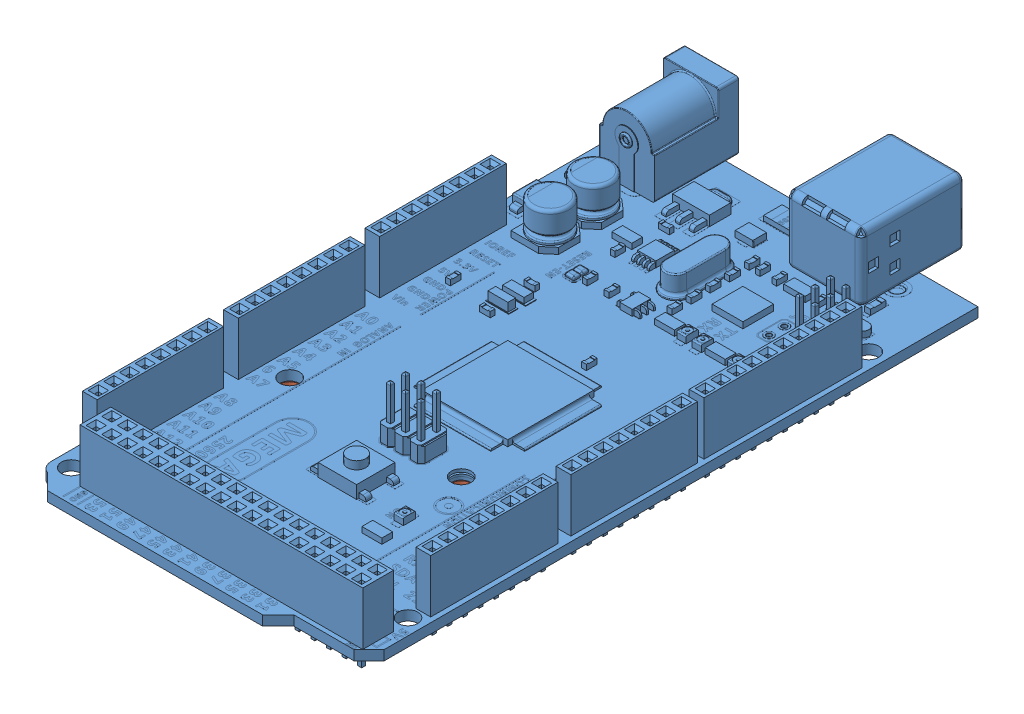
SolidWorks assembly ArduinoMegaAssembly, configuration Default. Lengths in mm.
Overall size (53.6 26.41 108.35).
2 component instances, 2 part files, 3 mates.
Components (placement in the parent):
- Arduino MEGA 2560 R3-1: Arduino MEGA 2560 R3 [Default] at (15.5804 57.3596 95.7334) size (53.6 14.61 108.35)
- ArduinoMegaHolder-1: ArduinoMegaHolder [Default] at (14.6304 55.7596 86.5284) x (1 0 0) z (0 -1 0) size (38.5 71.19 13.8)
Mates (geometry in assembly coordinates):
- Coincident1: coincident anti-aligned: plane of Arduino MEGA 2560 R3-1 through (15.5804 55.7596 95.7334) normal (0 -1 0); plane of ArduinoMegaHolder-1 through (14.6304 55.7596 86.5284) normal (0 1 0)
- Distance2: distance = 6 mm aligned: plane of ArduinoMegaHolder-1 through (-7.0196 50.7596 50.9334) normal (0 0 -1); plane of Arduino MEGA 2560 R3-1 through (-11.2196 55.7596 44.9334) normal (0 0 -1)
- Distance3: distance = 4.62 mm aligned: plane of ArduinoMegaHolder-1 through (-6.5996 55.7596 122.1234) normal (-1 0 0); plane of Arduino MEGA 2560 R3-1 through (-11.2196 55.7596 44.9334) normal (-1 0 0)
